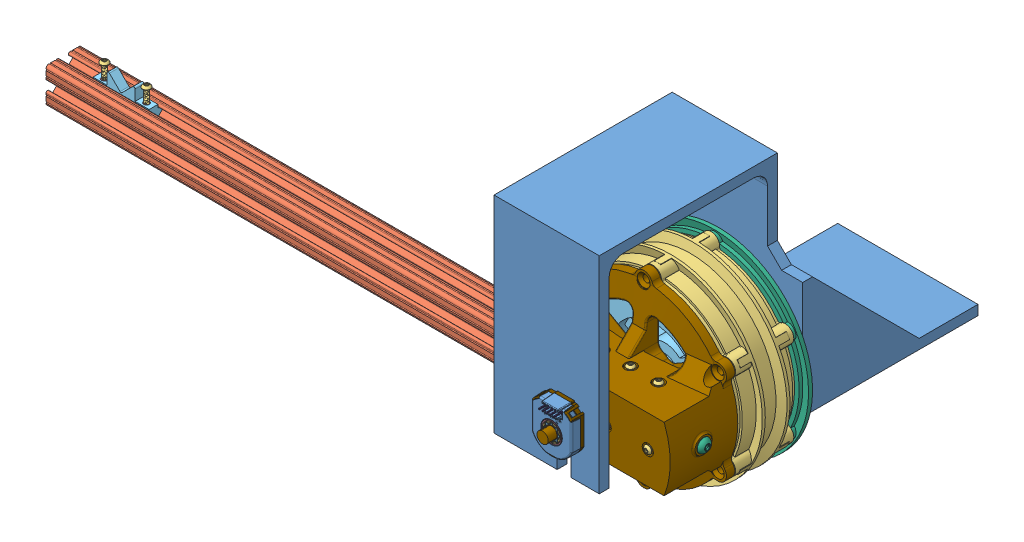
SolidWorks assembly torque_test, configuration Default. Lengths in mm.
Overall size (461.12 184.12 260.4).
82 component instances, 24 part files, 44 mates.
Components (placement in the parent):
- test_stand-2: test_stand [Default] at (3.6129 50.1777 -45.6114) size (100 147 245)
- M365 Nut-1: M365 Nut [Default] at (3.6129 80.1777 72.3886) x (1 0 0) z (0 1 0) size (23.5 10 23.5)
- M365-1: M365 [Default] at (3.6129 80.1777 115.3886) x (-1 0 0) z (0 0 -1) size (134.25 134.25 103.5)
  - M365 Rotor-1: M365 Rotor [Default] at origin size (134.25 134.25 41.5)
  - M365 Magnet-1: M365 Magnet [Default] at (0 -1.005 -1.5) size (11.29 3 30.5)
  - M365 Magnet-2: M365 Magnet [Default] at (-0.209 -0.9831 -1.5) x (0.978148 -0.207912 0) z (0 0 1) size (11.29 3 30.5)
  - M365 Magnet-3: M365 Magnet [Default] at (-0.4088 -0.9181 -1.5) x (0.913545 -0.406737 0) z (0 0 1) size (11.29 3 30.5)
  - M365 Magnet-4: M365 Magnet [Default] at (-0.5907 -0.8131 -1.5) x (0.809017 -0.587785 0) z (0 0 1) size (11.29 3 30.5)
  - M365 Magnet-5: M365 Magnet [Default] at (-0.7469 -0.6725 -1.5) x (0.669131 -0.743145 0) z (0 0 1) size (11.29 3 30.5)
  - M365 Magnet-6: M365 Magnet [Default] at (-0.8704 -0.5025 -1.5) x (0.5 -0.866025 0) z (0 0 1) size (11.29 3 30.5)
  - M365 Magnet-7: M365 Magnet [Default] at (-0.9558 -0.3106 -1.5) x (0.309017 -0.951057 0) z (0 0 1) size (11.29 3 30.5)
  - M365 Magnet-8: M365 Magnet [Default] at (-0.9995 -0.1051 -1.5) x (0.104528 -0.994522 0) z (0 0 1) size (11.29 3 30.5)
  - M365 Magnet-9: M365 Magnet [Default] at (-0.9995 0.1051 -1.5) x (-0.104528 -0.994522 0) z (0 0 1) size (11.29 3 30.5)
  - M365 Magnet-10: M365 Magnet [Default] at (-0.9558 0.3106 -1.5) x (-0.309017 -0.951057 0) z (0 0 1) size (11.29 3 30.5)
  - M365 Magnet-11: M365 Magnet [Default] at (-0.8704 0.5025 -1.5) x (-0.5 -0.866025 0) z (0 0 1) size (11.29 3 30.5)
  - M365 Magnet-12: M365 Magnet [Default] at (-0.7469 0.6725 -1.5) x (-0.669131 -0.743145 0) z (0 0 1) size (11.29 3 30.5)
  - M365 Magnet-13: M365 Magnet [Default] at (-0.5907 0.8131 -1.5) x (-0.809017 -0.587785 0) z (0 0 1) size (11.29 3 30.5)
  - M365 Magnet-14: M365 Magnet [Default] at (-0.4088 0.9181 -1.5) x (-0.913545 -0.406737 0) z (0 0 1) size (11.29 3 30.5)
  - M365 Magnet-15: M365 Magnet [Default] at (-0.209 0.9831 -1.5) x (-0.978148 -0.207912 0) z (0 0 1) size (11.29 3 30.5)
  - M365 Magnet-16: M365 Magnet [Default] at (0 1.005 -1.5) x (-1 0 0) z (0 0 1) size (11.29 3 30.5)
  - M365 Magnet-17: M365 Magnet [Default] at (0.209 0.9831 -1.5) x (-0.978148 0.207912 0) z (0 0 1) size (11.29 3 30.5)
  - M365 Magnet-18: M365 Magnet [Default] at (0.4088 0.9181 -1.5) x (-0.913545 0.406737 0) z (0 0 1) size (11.29 3 30.5)
  - M365 Magnet-19: M365 Magnet [Default] at (0.5907 0.8131 -1.5) x (-0.809017 0.587785 0) z (0 0 1) size (11.29 3 30.5)
  - M365 Magnet-20: M365 Magnet [Default] at (0.7469 0.6725 -1.5) x (-0.669131 0.743145 0) z (0 0 1) size (11.29 3 30.5)
  - M365 Magnet-21: M365 Magnet [Default] at (0.8704 0.5025 -1.5) x (-0.5 0.866025 0) z (0 0 1) size (11.29 3 30.5)
  - M365 Magnet-22: M365 Magnet [Default] at (0.9558 0.3106 -1.5) x (-0.309017 0.951057 0) z (0 0 1) size (11.29 3 30.5)
  - M365 Magnet-23: M365 Magnet [Default] at (0.9995 0.1051 -1.5) x (-0.104528 0.994522 0) z (0 0 1) size (11.29 3 30.5)
  - M365 Magnet-24: M365 Magnet [Default] at (0.9995 -0.1051 -1.5) x (0.104528 0.994522 0) z (0 0 1) size (11.29 3 30.5)
  - M365 Magnet-25: M365 Magnet [Default] at (0.9558 -0.3106 -1.5) x (0.309017 0.951057 0) z (0 0 1) size (11.29 3 30.5)
  - M365 Magnet-26: M365 Magnet [Default] at (0.8704 -0.5025 -1.5) x (0.5 0.866025 0) z (0 0 1) size (11.29 3 30.5)
  - M365 Magnet-27: M365 Magnet [Default] at (0.7469 -0.6725 -1.5) x (0.669131 0.743145 0) z (0 0 1) size (11.29 3 30.5)
  - M365 Magnet-28: M365 Magnet [Default] at (0.5907 -0.8131 -1.5) x (0.809017 0.587785 0) z (0 0 1) size (11.29 3 30.5)
  - M365 Magnet-29: M365 Magnet [Default] at (0.4088 -0.9181 -1.5) x (0.913545 0.406737 0) z (0 0 1) size (11.29 3 30.5)
  - M365 Magnet-30: M365 Magnet [Default] at (0.209 -0.9831 -1.5) x (0.978148 0.207912 0) z (0 0 1) size (11.29 3 30.5)
  - M365 Stator-1: M365 Stator [Default] at (0 0 -2.5) x (1 0 0) z (0 0 -1) size (105 105 103.5)
  - M365 Cap-1: M365 Cap [Default] at (0 0 21.5) size (134.25 134.25 12.37)
  - 5972K83_Ball Bearing-3: 5972K83_Ball Bearing [5972K83] at (0 0 25.625) size (32 32 9)
  - 5972K83_Ball Bearing-2: 5972K83_Ball Bearing [5972K83] at (0 0 -25.25) x (1 0 0) z (0 0 -1) size (32 32 9)
  - M365 Washer-1: M365 Washer [Default] at (0 0 34.625) x (-1 0 0) z (0 -1 0) size (22 2.75 22)
- torque_test_rotor_output-1: torque_test_rotor_output [Default] at (3.6129 80.1777 136.6386) size (123 134.25 78.15)
- rotor_output_ring-1: rotor_output_ring [Default] at (3.6129 80.1777 137.8886) x (1 0 0) z (0 1 0) size (114.5 2.5 114.5)
- CUI_DEVICES_CUI_DEVICES_AMT103-D0048-I8000-S-1: CUI_DEVICES_CUI_DEVICES_AMT103-D0048-I8000-S [Default] at (3.6129 80.1777 203.1586) x (-1 0 0) z (0 0 1) size (36.33 37.04 14.49)
  - CUI_DEVICES_AMT-Sleeve-REV-D(8 mm)-1: CUI_DEVICES_AMT-Sleeve-REV-D(8 mm) [Default] at (0 0 -2.42) x (0.999996 0.002864 0) z (0 0 1) size (10.79 10.79 7.8)
  - CUI_DEVICES_AMT-Hub-Top-REV-D1-1: CUI_DEVICES_AMT-Hub-Top-REV-D1 [Default] at (0 0 2.13) x (0.999996 0.002864 0) z (0 0 1) size (14 14 5.67)
  - CUI_DEVICES_AMT-Hub-Bottom-REV-B-1: CUI_DEVICES_AMT-Hub-Bottom-REV-B [Default] at (0 0 2.43) x (0.999998 -0.001942 0) z (0 0 1) size (17.3 17.3 3.2)
  - CUI_DEVICES_AMT10X-Shaft-Adaptor-REV-E-1: CUI_DEVICES_AMT10X-Shaft-Adaptor-REV-E [Default] at (0 0 0.03) x (0.999996 0.002864 0) z (0 0 1) size (11.8 11.8 7.8)
  - CUI_DEVICES_Receiver-board-1: CUI_DEVICES_Receiver-board [Default] at (72.2834 -20.351 3.03) x (-1 0 0) z (0 0 -1) size (26.5 26.62 0.41)
  - CUI_DEVICES_Rotor-board-REV F-1: CUI_DEVICES_Rotor-board-REV F [Default] at (0 0 2.13) x (0.807874 -0.589355 0) z (0 0 1) size (26 26 0.3)
  - CUI_DEVICES_Transmitter-board AMT10(AMT-103)-1: CUI_DEVICES_Transmitter-board AMT10(AMT-103) [Default] at (19.1596 -17.1102 1.22) x (-1 0 0) z (0 0 -1) size (26.63 29.61 12.1)
  - CUI_DEVICES_AMT-103-Base-REV-K(Default)-1: CUI_DEVICES_AMT-103-Base-REV-K(Default) [Default] at (0 0 -1) x (-1 0 0) z (0 0 -1) size (28.59 34.62 9.11)
  - CUI_DEVICES_AMT-103-Top-Cover-REV-I-1: CUI_DEVICES_AMT-103-Top-Cover-REV-I [Default] at (0 0 5.23) x (-1 0 0) z (0 0 -1) size (28.6 33.94 9.26)
- 1010_17_48_CL-1: 1010_17_48_CL [Default] at (-390.3791 80.1777 162.0886) x (0 0 1) z (-1 0 0) size (25.4 25.4 443.99)
- 92095A472_Button Head Hex Drive Screw-1: 92095A472_Button Head Hex Drive Screw [92095A472] at (48.6129 80.1777 186.2344) size (5.7 5.7 20.01)
- 94459A140_Brass Heat-Set Inserts for Plastic-1: 94459A140_Brass Heat-Set Inserts for Plastic [94459A140] at (48.6129 80.1777 176.0886) x (1 0 0) z (0 -1 0) size (4.77 6.11 4.77)
- 92095A472_Button Head Hex Drive Screw-2: 92095A472_Button Head Hex Drive Screw [92095A472] at (18.6129 80.1777 186.2344) size (5.7 5.7 20.01)
- 92095A472_Button Head Hex Drive Screw-3: 92095A472_Button Head Hex Drive Screw [92095A472] at (-11.3871 80.1777 186.2344) size (5.7 5.7 20.01)
- 92095A472_Button Head Hex Drive Screw-4: 92095A472_Button Head Hex Drive Screw [92095A472] at (-41.3871 80.1777 186.2344) size (5.7 5.7 20.01)
- 92095A472_Button Head Hex Drive Screw-6: 92095A472_Button Head Hex Drive Screw [92095A472] at (33.6129 104.3235 162.0886) x (1 0 0) z (0 1 0) size (5.7 5.7 20.01)
- 92095A472_Button Head Hex Drive Screw-7: 92095A472_Button Head Hex Drive Screw [92095A472] at (13.6129 104.3235 162.0886) x (1 0 0) z (0 1 0) size (5.7 5.7 20.01)
- 92095A472_Button Head Hex Drive Screw-8: 92095A472_Button Head Hex Drive Screw [92095A472] at (-6.3871 104.3235 162.0886) x (1 0 0) z (0 1 0) size (5.7 5.7 20.01)
- 92095A472_Button Head Hex Drive Screw-9: 92095A472_Button Head Hex Drive Screw [92095A472] at (-26.3871 104.3235 162.0886) x (1 0 0) z (0 1 0) size (5.7 5.7 20.01)
- 92095A472_Button Head Hex Drive Screw-10: 92095A472_Button Head Hex Drive Screw [92095A472] at (33.6129 56.0319 162.0886) x (1 0 0) z (0 -1 0) size (5.7 5.7 20.01)
- 92095A472_Button Head Hex Drive Screw-11: 92095A472_Button Head Hex Drive Screw [92095A472] at (13.6129 56.0319 162.0886) x (1 0 0) z (0 -1 0) size (5.7 5.7 20.01)
- 92095A472_Button Head Hex Drive Screw-12: 92095A472_Button Head Hex Drive Screw [92095A472] at (-6.3871 56.0319 162.0886) x (1 0 0) z (0 -1 0) size (5.7 5.7 20.01)
- 92095A472_Button Head Hex Drive Screw-13: 92095A472_Button Head Hex Drive Screw [92095A472] at (-26.3871 56.0319 162.0886) x (1 0 0) z (0 -1 0) size (5.7 5.7 20.01)
- 94459A140_Brass Heat-Set Inserts for Plastic-2: 94459A140_Brass Heat-Set Inserts for Plastic [94459A140] at (33.6129 94.1777 162.0886) size (4.77 6.11 4.77)
- 94459A140_Brass Heat-Set Inserts for Plastic-3: 94459A140_Brass Heat-Set Inserts for Plastic [94459A140] at (18.6129 80.1777 176.0886) x (1 0 0) z (0 -1 0) size (4.77 6.11 4.77)
- 94459A140_Brass Heat-Set Inserts for Plastic-4: 94459A140_Brass Heat-Set Inserts for Plastic [94459A140] at (-11.3871 80.1777 176.0886) x (1 0 0) z (0 -1 0) size (4.77 6.11 4.77)
- 94459A140_Brass Heat-Set Inserts for Plastic-5: 94459A140_Brass Heat-Set Inserts for Plastic [94459A140] at (-41.3871 80.1777 176.0886) x (1 0 0) z (0 -1 0) size (4.77 6.11 4.77)
- 94459A140_Brass Heat-Set Inserts for Plastic-6: 94459A140_Brass Heat-Set Inserts for Plastic [94459A140] at (13.6129 94.1777 162.0886) size (4.77 6.11 4.77)
- 94459A140_Brass Heat-Set Inserts for Plastic-7: 94459A140_Brass Heat-Set Inserts for Plastic [94459A140] at (-6.3871 94.1777 162.0886) size (4.77 6.11 4.77)
- 94459A140_Brass Heat-Set Inserts for Plastic-8: 94459A140_Brass Heat-Set Inserts for Plastic [94459A140] at (-26.3871 94.1777 162.0886) size (4.77 6.11 4.77)
- 94459A140_Brass Heat-Set Inserts for Plastic-9: 94459A140_Brass Heat-Set Inserts for Plastic [94459A140] at (33.6129 60.4666 162.0886) size (4.77 6.11 4.77)
- 94459A140_Brass Heat-Set Inserts for Plastic-10: 94459A140_Brass Heat-Set Inserts for Plastic [94459A140] at (13.6129 60.4666 162.0886) size (4.77 6.11 4.77)
- 94459A140_Brass Heat-Set Inserts for Plastic-11: 94459A140_Brass Heat-Set Inserts for Plastic [94459A140] at (-6.3871 60.4666 162.0886) size (4.77 6.11 4.77)
- 94459A140_Brass Heat-Set Inserts for Plastic-12: 94459A140_Brass Heat-Set Inserts for Plastic [94459A140] at (-26.3871 60.4666 162.0886) size (4.77 6.11 4.77)
- rope_holder-1: rope_holder [Default] at (-346.3871 85.1679 162.0886) x (0 0 1) z (-1 0 0) size (14.5 16.34 40)
- 94459A140_Brass Heat-Set Inserts for Plastic-13: 94459A140_Brass Heat-Set Inserts for Plastic [94459A140] at (-361.3871 87.2179 162.0886) size (4.77 6.11 4.77)
- 92095A472_Button Head Hex Drive Screw-14: 92095A472_Button Head Hex Drive Screw [92095A472] at (-361.3871 104.3235 162.0886) x (1 0 0) z (0 1 0) size (5.7 5.7 20.01)
- 92095A472_Button Head Hex Drive Screw-15: 92095A472_Button Head Hex Drive Screw [92095A472] at (-331.3871 104.3235 162.0886) x (-1 0 0) z (0 1 0) size (5.7 5.7 20.01)
- 94459A140_Brass Heat-Set Inserts for Plastic-14: 94459A140_Brass Heat-Set Inserts for Plastic [94459A140] at (-331.3871 92.9291 162.0886) x (-1 0 0) z (0 0 1) size (4.77 6.11 4.77)
- 92949A433_18-8 Stainless Steel Button Head Hex Drive Screw-1: 92949A433_18-8 Stainless Steel Button Head Hex Drive Screw [92949A433] at (54.4369 80.1777 162.0886) x (0 0 1) z (1 0 0) size (9.6 9.6 29.08)
Mates (geometry in assembly coordinates):
- Concentric1: concentric aligned: cylinder of torque_test_rotor_output-1 through (3.6129 141.1777 136.6386) axis (0 0 1) radius 2.5; cylinder of M365-1/M365 Rotor-1 through (3.6129 141.1777 130.1386) axis (0 0 1) radius 1.5
- Concentric2: concentric aligned: cylinder of torque_test_rotor_output-1 through (3.6129 19.1777 136.6386) axis (0 0 1) radius 2.5; cylinder of M365-1/M365 Rotor-1 through (3.6129 19.1777 130.1386) axis (0 0 1) radius 1.5
- Parallel15: parallel aligned: plane of M365 Nut-1 through (3.6129 80.1777 72.3886) normal (1 0 0)
- Concentric40: concentric aligned: cylinder of M365 Nut-1 through (3.6129 80.1777 62.3886) axis (0 0 1) radius 6; cylinder of M365-1/M365 Stator-1 through (3.6129 80.1777 63.6386) axis (0 0 1) radius 6
- Concentric41: concentric anti-aligned: cylinder of torque_test_rotor_output-1 through (3.6129 80.1777 142.6386) axis (0 0 -1) radius 57.25; cylinder of rotor_output_ring-1 through (3.6129 80.1777 135.3886) axis (0 0 1) radius 54.75
- Coincident65: coincident anti-aligned: plane of torque_test_rotor_output-1 through (3.6129 80.1777 137.8886) normal (0 0 -1); plane of rotor_output_ring-1 through (3.6129 80.1777 137.8886) normal (0 0 1)
- Parallel33: parallel aligned: plane of rotor_output_ring-1 through (3.6129 80.1777 137.8886) normal (1 0 0)
- Coincident67: coincident aligned: cone of M365-1/M365 Rotor-1 through (3.6129 80.1777 136.1386) axis (0 0 -1); cone of rotor_output_ring-1 through (3.6129 80.1777 135.3886) axis (0 0 -1)
- Parallel34: parallel anti-aligned: plane of CUI_DEVICES_CUI_DEVICES_AMT103-D0048-I8000-S-1 through (3.6129 80.1777 203.1586) normal (-1 0 0)
- Concentric44: concentric aligned: cylinder of torque_test_rotor_output-1 through (48.6129 80.1777 136.6376) axis (0 0 1) radius 1.975; cylinder of 92095A472_Button Head Hex Drive Screw-1 through (48.6129 80.1777 186.2344) axis (0 0 1) radius 2.85
- Coincident69: coincident anti-aligned: plane of torque_test_rotor_output-1 through (3.6129 67.4777 136.6376) normal (0 1 0); plane of 1010_17_48_CL-1 through (53.6129 67.4777 168.4217) normal (0 -1 0)
- Coincident70: coincident anti-aligned: plane of torque_test_rotor_output-1 through (3.6129 80.1777 174.7886) normal (0 0 -1); plane of 1010_17_48_CL-1 through (53.6129 70.6273 174.7886) normal (0 0 1)
- Parallel35: parallel aligned: plane of 3205-1 through (52.366 85.2704 172.1978) normal (1 0 0)
- Parallel36: parallel aligned: plane of 92095A472_Button Head Hex Drive Screw-1 through (48.6129 80.1777 186.2344) normal (1 0 0)
- Concentric47: concentric anti-aligned: cylinder of torque_test_rotor_output-1 through (33.6129 147.3037 162.0886) axis (0 -1 0) radius 1.975; cylinder of 92095A472_Button Head Hex Drive Screw-6 through (33.6129 104.3235 162.0886) axis (0 1 0) radius 2.85
- Parallel37: parallel aligned: plane of 92095A472_Button Head Hex Drive Screw-6 through (33.6129 104.3235 162.0886) normal (1 0 0)
- Parallel38: parallel aligned: plane of 3205-5 through (37.366 90.2869 156.9959) normal (1 0 0)
- Concentric48: concentric aligned: cylinder of M365-1/M365 Stator-1 through (3.6129 80.1777 63.6386) axis (0 0 1) radius 6; cylinder of test_stand2-1 through (3.6129 80.1777 -45.6124) axis (0 0 1) radius 6
- Coincident76: coincident anti-aligned: plane of M365 Nut-1 through (3.6129 80.1777 72.3886) normal (0 0 1); plane of test_stand2-1 through (53.6129 197.1777 72.3886) normal (0 0 -1)
- Coincident77: coincident anti-aligned: plane of M365-1/M365 Washer-1 through (3.6129 80.1777 79.3886) normal (0 0 -1); plane of test_stand-2 through (3.6129 50.1777 79.3886) normal (0 0 1)
- Coincident85: coincident anti-aligned: plane of CUI_DEVICES_CUI_DEVICES_AMT103-D0048-I8000-S-1/CUI_DEVICES_AMT-103-Base-REV-K(Default)-1 through (3.6129 80.1777 199.3886) normal (0 0 -1); plane of test_stand-2 through (3.6129 50.1777 199.3886) normal (0 0 1)
- Perpendicular1: perpendicular: plane of CUI_DEVICES_CUI_DEVICES_AMT103-D0048-I8000-S-1/CUI_DEVICES_AMT-103-Top-Cover-REV-I-1 through (17.9129 74.1978 201.8886) normal (0.999848 0 0.017452); plane of test_stand-2 through (3.6129 50.1777 -45.6114) normal (0 -1 0)
- Concentric49: concentric anti-aligned: cylinder of torque_test_rotor_output-1 through (3.6129 80.1777 214.7886) axis (0 0 -1) radius 4; cylinder of CUI_DEVICES_CUI_DEVICES_AMT103-D0048-I8000-S-1/CUI_DEVICES_AMT-Sleeve-REV-D(8 mm)-1 through (3.6129 80.1777 200.7386) axis (0 0 1) radius 4
- Concentric50: concentric anti-aligned: cylinder of torque_test_rotor_output-1 through (48.6129 80.1777 136.6376) axis (0 0 1) radius 1.975; cylinder of 94459A140_Brass Heat-Set Inserts for Plastic-1 through (48.6129 80.1777 176.0886) axis (0 0 -1) radius 1.95
- Coincident86: coincident aligned: plane of torque_test_rotor_output-1 through (48.6129 80.1777 181.7886) normal (0 0 1); plane of 94459A140_Brass Heat-Set Inserts for Plastic-1 through (50.9629 80.1777 181.7886) normal (0 0 1)
- Parallel39: parallel aligned: plane of 94459A140_Brass Heat-Set Inserts for Plastic-1 through (48.6129 80.1777 176.0886) normal (1 0 0)
- Concentric51: concentric aligned: cylinder of torque_test_rotor_output-1 through (33.6129 147.3037 162.0886) axis (0 -1 0) radius 1.975; cylinder of 94459A140_Brass Heat-Set Inserts for Plastic-2 through (33.6129 94.1777 162.0886) axis (0 -1 0) radius 1.95
- Coincident88: coincident aligned: plane of torque_test_rotor_output-1 through (33.6129 99.8777 162.0886) normal (0 1 0); plane of 94459A140_Brass Heat-Set Inserts for Plastic-2 through (35.9629 99.8777 162.0886) normal (0 1 0)
- Parallel40: parallel aligned: plane of 94459A140_Brass Heat-Set Inserts for Plastic-2 through (33.6129 94.1777 162.0886) normal (1 0 0)
- Coincident90: coincident anti-aligned: plane of 1010_17_48_CL-1 through (53.6129 84.6735 163.7067) normal (0 1 0); plane of 92095A472_Button Head Hex Drive Screw-6 through (33.6129 84.6735 162.0886) normal (0 -1 0)
- Coincident91: coincident anti-aligned: plane of 1010_17_48_CL-1 through (53.6129 78.5596 166.5844) normal (0 0 1); plane of 92095A472_Button Head Hex Drive Screw-1 through (48.6129 80.1777 166.5844) normal (0 0 -1)
- Coincident92: coincident anti-aligned: plane of 1010_17_48_CL-1 through (53.6129 90.6679 155.6138) normal (0 -1 0); plane of rope_holder-1 through (-366.3871 90.6679 158.8886) normal (0 1 0)
- Width1: width anti-aligned: plane of 1010_17_48_CL-1 through (53.6129 86.5108 174.7886) normal (0 0 1); plane of 1010_17_48_CL-1 through (53.6129 89.7281 149.3886) normal (0 0 -1); plane of rope_holder-1 through (-366.3871 92.9179 158.8886) normal (0 0 -1); plane of rope_holder-1 through (-366.3871 90.6679 165.2886) normal (0 0 1)
- Distance1: distance = 350 mm anti-aligned: plane of rope_holder-1 through (-346.3871 85.1679 162.0886) normal (-1 0 0); plane of torque_test_rotor_output-1 through (3.6129 80.1777 136.6386) normal (1 0 0)
- Coincident94: coincident aligned: plane of rope_holder-1 through (-366.3871 92.9179 165.2886) normal (0 1 0); plane of 94459A140_Brass Heat-Set Inserts for Plastic-13 through (-359.0371 92.9179 162.0886) normal (0 1 0)
- Concentric52: concentric anti-aligned: cylinder of rope_holder-1 through (-361.3871 85.1679 162.0886) axis (0 1 0) radius 1.975; cylinder of 94459A140_Brass Heat-Set Inserts for Plastic-13 through (-361.3871 87.2179 162.0886) axis (0 -1 0) radius 1.95
- Parallel42: parallel aligned: plane of 94459A140_Brass Heat-Set Inserts for Plastic-13 through (-361.3871 87.2179 162.0886) normal (1 0 0)
- Concentric53: concentric aligned: cylinder of rope_holder-1 through (-361.3871 85.1679 162.0886) axis (0 1 0) radius 1.975; cylinder of 92095A472_Button Head Hex Drive Screw-14 through (-361.3871 104.3235 162.0886) axis (0 1 0) radius 2.85
- Coincident97: coincident anti-aligned: plane of 1010_17_48_CL-1 through (53.6129 84.6735 163.7067) normal (0 1 0); plane of 92095A472_Button Head Hex Drive Screw-14 through (-361.3871 84.6735 162.0886) normal (0 -1 0)
- Parallel43: parallel aligned: plane of 92095A472_Button Head Hex Drive Screw-14 through (-361.3871 104.3235 162.0886) normal (1 0 0)
- Coincident98: coincident anti-aligned: plane of torque_test_rotor_output-1 through (53.6129 80.1777 136.6376) normal (-1 0 0); plane of 1010_17_48_CL-1 through (53.6129 70.1193 149.3886) normal (1 0 0)
- Concentric54: concentric aligned: cylinder of torque_test_rotor_output-1 through (-57.3881 80.1777 162.0886) axis (1 0 0) radius 3.15; cylinder of 92949A433_18-8 Stainless Steel Button Head Hex Drive Screw-1 through (68.6609 80.1777 162.0886) axis (1 0 0) radius 4.8006
- Coincident99: coincident anti-aligned: plane of torque_test_rotor_output-1 through (65.6129 80.1777 162.0886) normal (1 0 0); plane of 92949A433_18-8 Stainless Steel Button Head Hex Drive Screw-1 through (65.6129 75.3771 162.0886) normal (-1 0 0)
- Parallel45: parallel aligned: plane of 92949A433_18-8 Stainless Steel Button Head Hex Drive Screw-1 through (54.4369 80.1777 162.0886) normal (0 0 1)
